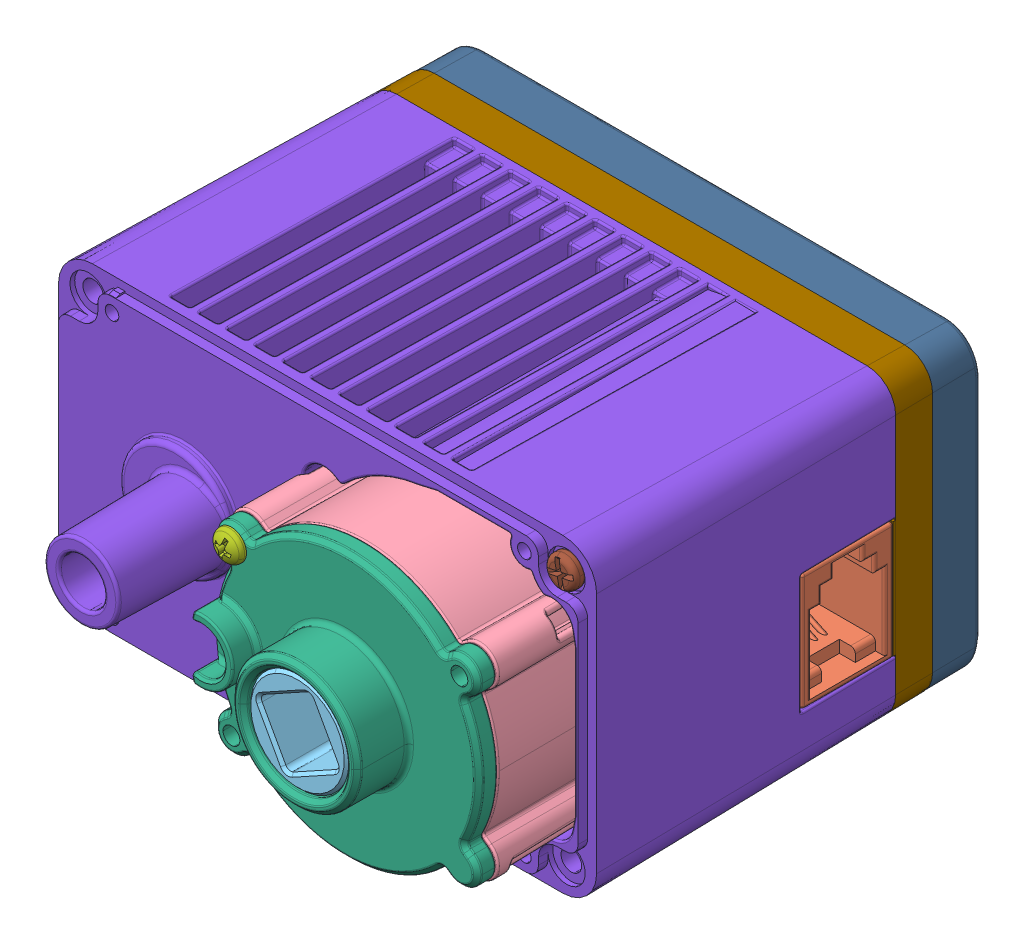
SolidWorks assembly V5 Smart Motor (276-4840) no cap, configuration Default. Lengths in mm.
20 component instances, 12 part files, 0 mates.
Components (placement in the parent):
- V5 Smart Motor (276-4840).step-1: V5 Smart Motor (276-4840).step [Default] at origin size (59.01 35.33 59.91)
  - 276-4840-900 Rev6_Instruction.step-1: 276-4840-900 Rev6_Instruction.step [Default] at (-14.3 0 -17.2) size (52.79 15.94 38.15) (hidden)
    - 276-4840-901 Rev6.step-1: 276-4840-901 Rev6.step [Default] at (10.75 -10.05 17.8) x (-1 0 0) z (0 0 1) size (49.9 1.6 38.15) (hidden)
    - 276-4840-902 Rev2.step-1: 276-4840-902 Rev2.step [Default] at (31.25 -9.25 6.2) x (0 0 -1) z (0 -1 0) size (10.35 11.39 15.94) (hidden)
    - 276-4840-022 Rev4.step-1: 276-4840-022 Rev4.step [Default] at (31.25 -9.25 6.2) x (0 0 -1) z (1 0 0) size (10.26 9.1 5.51) (hidden)
  - 276-4840-110 Rev10_Instruction.step-1: 276-4840-110 Rev10_Instruction.step [Default] at (12.7 0 14.7) size (35.33 35.33 31.1) (hidden)
    - 276-4840-061 Rev7_Ring_Gear_Fixed01 .6 Rev3.step-1: 276-4840-061 Rev7_Ring_Gear_Fixed01 .6 Rev3.step [Default] at origin size (28.79 28.39 24.6) (hidden)
    - 276-4840-018 Rev6.step-1: 276-4840-018 Rev6.step [Default] at (0 0 6.7) x (-0.483174 0.875524 0) z (0 0 1) size (26 26 12.3) (hidden)
    - 276-4840-059 Rev2.step-1: 276-4840-059 Rev2.step [Default] at (0 0 10.3) size (28.4 28.4 8.5) (hidden)
    - 276-4840-062 Rev1.step-1: 276-4840-062 Rev1.step [Default] at (-12.1353 8.8168 12.3) x (0.956835 -0.290632 0) z (-0.290632 -0.956835 0) size (3.2 6.56 3.2) (hidden)
    - 276-4840-062 Rev1.step-2: 276-4840-062 Rev1.step [Default] at (12.1353 8.8168 12.3) x (0.978427 0.206591 0) z (0.206591 -0.978427 0) size (3.2 6.56 3.2) (hidden)
    - 276-4840-062 Rev1.step-3: 276-4840-062 Rev1.step [Default] at (-12.1353 -8.8168 12.3) x (0.72563 0.688086 0) z (0.688086 -0.72563 0) size (3.2 6.56 3.2) (hidden)
  - 276-4840-001 Rev38.step-1: 276-4840-001 Rev38.step [Default] at origin size (57.3 33 46.9) (hidden)
  - 276-4840-005 Rev27.step-1: 276-4840-005 Rev27.step [Default] at (0 0 -17.95) size (56.17 31.87 12.9) (hidden)
  - 276-4840-004 Rev16.step-1: 276-4840-004 Rev16.step [Default] at (0 0 -19.2) size (56.01 31.71 9.21) (hidden)
  - 276-4840-009 Rev3.step-1: 276-4840-009 Rev3.step [Default] at (25.45 13.5 15.7) x (0.19987 -0.979823 0) z (-0.979823 -0.19987 0) size (3.4 41.31 4.34) (hidden)
  - 276-4840-009 Rev3.step-2: 276-4840-009 Rev3.step [Default] at (-25.45 -13.5 15.7) x (-0.998855 0.047836 0) z (0.047836 0.998855 0) size (3.4 41.31 4.34) (hidden)
  - 276-4840-009 Rev3.step-3: 276-4840-009 Rev3.step [Default] at (25.45 -13.5 15.7) x (-0.975374 0.220559 0) z (0.220559 0.975374 0) size (3.4 41.31 4.34) (hidden)
  - 276-4840-009 Rev3.step-4: 276-4840-009 Rev3.step [Default] at (-25.45 13.5 15.7) x (-0.922256 0.38658 0) z (0.38658 0.922256 0) size (3.4 41.31 4.34) (hidden)
  - 276-4840-025 Rev19.step-1: 276-4840-025 Rev19.step [Default] at (12.7 0 -22.63) x (-0.993315 0.115437 0) z (0 0 1) size (14.82 14.83 35.18) (hidden)
